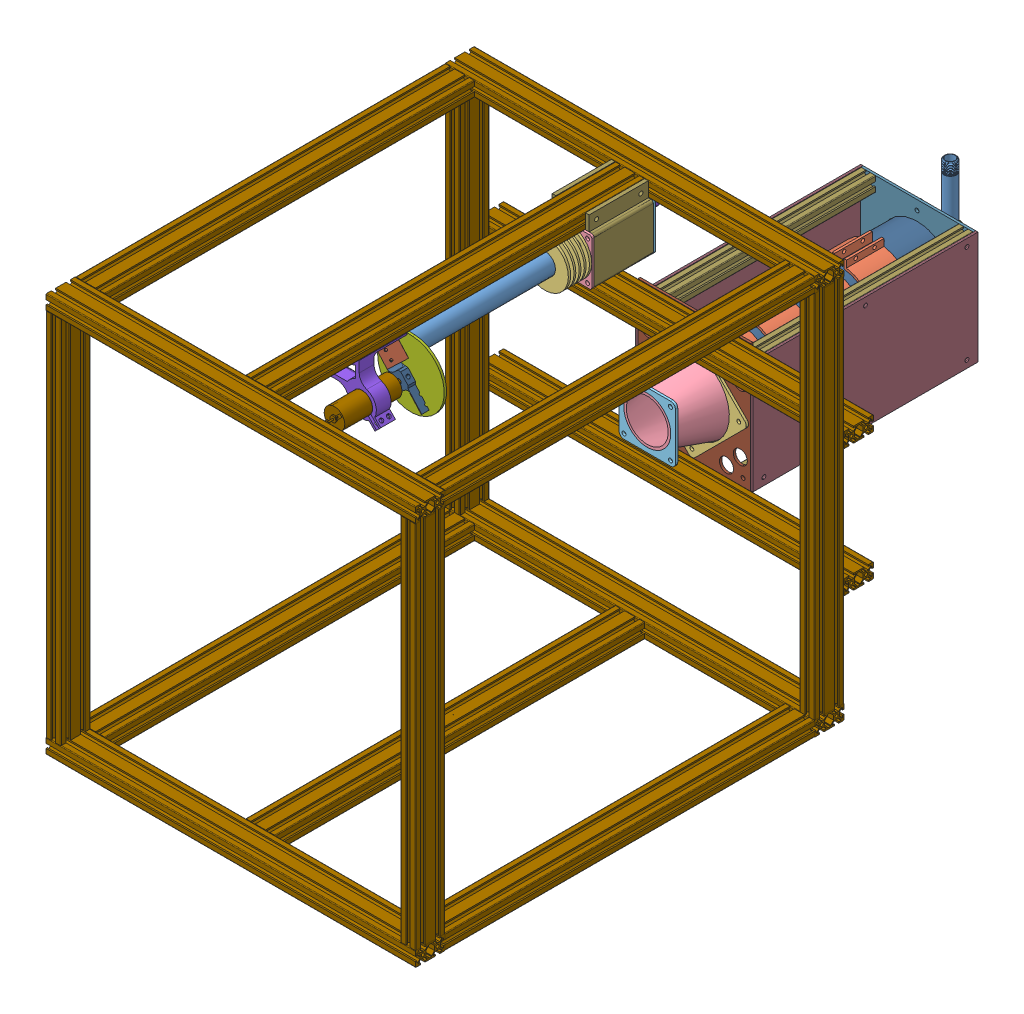
SolidWorks assembly extruder 1 assembly, configuration Default. Lengths in mm.
Overall size (500 540 979.81).
58 component instances, 30 part files, 85 mates.
Components (placement in the parent):
- extruder barrel_rev01-1: extruder barrel_rev01 [Default] at (188.8223 217.5446 43.8354) size (28.57 28.57 304.8)
- nozzle_rev01-1: nozzle_rev01 [Default] at (188.8223 217.5446 329.5854) size (28.57 28.57 31.75)
- barrel lock-1: barrel lock [Default] at (188.8223 217.5446 154.9604) x (-0.997738 -0.067218 0) z (0.067218 -0.997738 0) size (63.5 31.75 63.5)
- barrel lock mount-1: barrel lock mount [Default] at (188.8223 217.5446 120.0354) x (1 0 0) z (0 -1 0) size (63.5 3.17 63.5)
- thrust bearing plate-1: thrust bearing plate [Default] at (188.8223 217.5446 40.0354) x (1 0 0) z (0 1 0) size (63.5 3.17 63.5)
- 5909K310_THRUST NEEDLE-ROLLER BEARING-1: 5909K310_THRUST NEEDLE-ROLLER BEARING [5909K31] at (188.8223 217.5446 42.0304) x (1 0 0) z (0 -1 0) size (23.81 19.84 23.81)
- 5909K440_THRUST NEEDLE-ROLLER BEARING-1: 5909K440_THRUST NEEDLE-ROLLER BEARING [5909K44] at (188.8223 217.5446 41.0382) x (0 0 -1) z (0.082579 0.996584 0) size (0.81 23.81 23.81)
- 5909K440_THRUST NEEDLE-ROLLER BEARING-2: 5909K440_THRUST NEEDLE-ROLLER BEARING [5909K44] at (188.8223 217.5446 43.8354) x (0 0 -1) z (1 0 0) size (0.81 23.81 23.81)
- screw standin-1: screw standin [Default] at (188.8223 217.5446 310.5354) x (1 0 0) z (0 1 0) size (19.55 342.9 19.55)
- 500mm 2040-1: 500mm 2040 [Default] at (188.8223 259.2946 540.0354) x (0 -1 0) z (0 0 1) size (20 40 500)
- 500mm 2040-2: 500mm 2040 [Default] at (-61.3618 259.2946 560.0354) x (0 1 0) z (-1 0 0) size (20 40 500)
- 500mm 2040-3: 500mm 2040 [Default] at (-51.3618 249.2946 560.0354) x (1 0 0) z (0 1 0) size (20 40 500)
- 500mm 2040-4: 500mm 2040 [Default] at (428.6382 -250.7054 560.0354) x (1 0 0) z (0 -1 0) size (20 40 500)
- 500mm 2040-5: 500mm 2040 [Default] at (-61.3618 -260.7054 560.0354) x (0 1 0) z (-1 0 0) size (20 40 500)
- 500mm 2040-6: 500mm 2040 [Default] at (418.6382 259.2946 540.0354) x (0 1 0) z (0 0 1) size (20 40 500)
- 500mm 2040-7: 500mm 2040 [Default] at (-41.3618 259.2946 540.0354) x (0 1 0) z (0 0 1) size (20 40 500)
- 500mm 2040-8: 500mm 2040 [Default] at (418.6382 -260.7054 540.0354) x (0 1 0) z (0 0 1) size (20 40 500)
- 500mm 2040-9: 500mm 2040 [Default] at (-41.3618 -260.7054 540.0354) x (0 -1 0) z (0 0 1) size (20 40 500)
- 500mm 2040-10: 500mm 2040 [Default] at (-61.3618 -260.7054 20.0354) x (0 1 0) z (-1 0 0) size (20 40 500)
- 500mm 2040-11: 500mm 2040 [Default] at (-61.3618 259.2946 20.0354) x (0 -1 0) z (-1 0 0) size (20 40 500)
- 500mm 2040-12: 500mm 2040 [Default] at (-51.3618 249.2946 20.0354) x (-1 0 0) z (0 1 0) size (20 40 500)
- 500mm 2040-13: 500mm 2040 [Default] at (428.6382 249.2946 20.0354) x (1 0 0) z (0 1 0) size (20 40 500)
- 500mm 2040-14: 500mm 2040 [Default] at (188.8164 -260.7054 540.0354) x (0 -1 0) z (0 0 1) size (20 40 500)
- dryer stand alone-1: dryer stand alone [Default] at (381.6192 -132.2091 21.3365) x (0 1 0) z (-1 0 0) size (209.74 423.31 158.7)
  - tube-1: tube [Default] at (103.5422 61.3012 185.6839) size (164.34 304.8 101.6)
  - flange rev01-1: flange rev01 [Default] at (103.5422 61.3012 185.6839) x (-1 0 0) z (0 0 -1) size (192.4 3.17 152.4)
  - HFS5-2020-299-1: HFS5-2020-299 [Default] at (169.7422 63.9262 119.4839) x (-1 0 0) z (0 -1 0) size (20 20 298.45)
  - HFS5-2020-299-2: HFS5-2020-299 [Default] at (37.3422 63.9262 119.4839) x (-1 0 0) z (0 -1 0) size (20 20 298.45)
  - HFS5-2020-299-3: HFS5-2020-299 [Default] at (169.7422 63.9262 251.8839) x (-1 0 0) z (0 -1 0) size (20 20 298.45)
  - HFS5-2020-299-4: HFS5-2020-299 [Default] at (37.3422 363.4762 251.8839) x (-1 0 0) z (0 1 0) size (20 20 298.45)
  - side plate 1_16-1: side plate 1_16 [Default] at (103.5422 213.7012 263.4587) x (-1 0 0) z (0 0 -1) size (152.4 304.8 1.57)
  - side plate 1_16-2: side plate 1_16 [Default] at (103.5422 213.7012 265.0335) x (-1 0 0) z (0 0 -1) size (152.4 304.8 1.57)
  - flange rev02-1: flange rev02 [Default] at (103.5422 362.9262 185.6839) x (-1 0 0) z (0 0 -1) size (152.4 3.17 152.4)
  - top cover-1: top cover [Default] at (103.5422 369.2762 185.6839) x (-0.707107 0 -0.707107) z (0 -1 0) size (107.76 107.76 3.17)
  - 4452K413_TYPE 316 STAINLESS STL THREADED PIPE FITTING-2: 4452K413_TYPE 316 STAINLESS STL THREADED PIPE FITTING [4452K413] at (103.5422 407.8982 185.6839) x (-1 0 0) z (0 0 1) size (37.28 37.03 30.11)
  - 4548K159_STD-WALL TYPE 316-316L SS THRD PIPE NIPPLE-1: 4548K159_STD-WALL TYPE 316-316L SS THRD PIPE NIPPLE [4548K159] at (103.5422 292.6762 185.6839) x (0 1 0) z (0 0 1) size (203.35 17.91 17.78)
  - 4464K498_TYPE 304 STAINLESS STL THREADED PIPE FITTING-1: 4464K498_TYPE 304 STAINLESS STL THREADED PIPE FITTING [4464K498] at (103.5422 180.2482 185.6839) x (-0.837169 0 -0.546944) z (0 1 0) size (25.91 25.91 21.03)
  - 4548K145_STD-WALL TYPE 316-316L SS THRD PIPE NIPPLE-2: 4548K145_STD-WALL TYPE 316-316L SS THRD PIPE NIPPLE [4548K145] at (161.6142 407.8982 185.6839) x (1 0 0) z (0 -0.851872 -0.523749) size (89.04 17.99 18.06)
  - heater band-1: heater band [Default] at (103.5422 257.8762 185.6839) size (116.47 50.8 107.95)
  - heater band-2: heater band [Default] at (103.5422 132.2762 185.6839) size (116.47 50.8 107.95)
  - heater band-3: heater band [Default] at (103.5422 69.4762 185.6839) size (116.47 50.8 107.95)
  - heater band-4: heater band [Default] at (103.5422 195.0762 185.6839) size (116.47 50.8 107.95)
  - bottom cover-1: bottom cover [Default] at (103.6306 61.3012 185.6839) x (-0.707107 0 -0.707107) z (0 -1 0) size (107.76 107.76 3.17)
  - nozzle reduction-1: nozzle reduction [Default] at (103.6306 61.3012 185.6839) x (-0.837169 0 -0.546944) z (-0.546944 0 0.837169) size (101.6 63.5 101.6)
  - 2.5 in bracket-1: 2.5 in bracket [Default] at (103.6306 -2.1988 185.6839) size (76.2 3.17 76.2)
  - side plate 1_16-7: side plate 1_16 [Default] at (103.5422 213.7012 107.9091) size (152.4 304.8 1.57)
  - side plate 1_16-8: side plate 1_16 [Default] at (103.5422 213.7012 106.3343) size (152.4 304.8 1.57)
  - 9157K150_STD-WALL 304-304L SS THRD ONE END PIPE NIPPLE-1: 9157K150_STD-WALL 304-304L SS THRD ONE END PIPE NIPPLE [9157K15] at (103.5422 378.8012 152.0289) x (0 1 0) z (-0.332767 0 0.943009) size (25.49 27.89 27.84)
  - 9157K150_STD-WALL 304-304L SS THRD ONE END PIPE NIPPLE-2: 9157K150_STD-WALL 304-304L SS THRD ONE END PIPE NIPPLE [9157K15] at (103.5422 378.8012 219.3389) x (0 1 0) z (-0.546944 0 0.837169) size (25.49 27.89 27.84)
- pelletizer plate-1: pelletizer plate [Default] at (188.8223 217.5446 361.3354) x (-1 0 0) z (0 -1 0) size (90.17 3.17 90.52)
- pelletizer plate mount-1: pelletizer plate mount [Default] at (188.8223 244.2946 361.3354) x (1 0 0) z (0 -1 0) size (90.17 65 92.21)
- 3262_1-2: 3262_1 [Default] at (212.8568 202.1389 463.8354) x (-0.745096 -0.666957 0) z (0 0 -1) size (28 28 106.2)
- blade wheel-1: blade wheel [Default] at (212.8568 202.1389 366.6354) x (-0.666957 0.745096 0) z (0.745096 0.666957 0) size (76.2 10 20)
- blade fin-1: blade fin [Default] at (229.121 181.0645 369.3692) x (0.570777 0.510919 0.642788) z (-0.666957 0.745096 0) size (23.8 0.5 23.1)
- blade fin-2: blade fin [Default] at (196.3535 222.9985 368.9862) x (-0.570777 -0.510919 0.642788) z (-0.666957 0.745096 0) size (23.8 0.5 23.1)
- hopper rev02-2: hopper rev02 [Default] at (188.8223 217.5446 120.0354) x (1 0 0) z (0 1 0) size (63.5 80 83.5)
- 500mm 2040-16: 500mm 2040 [Default] at (-61.3618 57.5332 -19.9646) x (0 -1 0) z (-1 0 0) size (20 40 500)
- 500mm 2040-17: 500mm 2040 [Default] at (438.6382 -114.8668 -19.9646) x (0 -1 0) z (1 0 0) size (20 40 500)
Mates (geometry in assembly coordinates):
- Concentric1: concentric anti-aligned: cylinder of extruder barrel_rev01-1 through (188.8223 217.5446 329.5854) axis (0 0 1) radius 11.1125; cylinder of nozzle_rev01-1 through (188.8223 217.5446 348.6354) axis (0 0 -1) radius 11.1125
- Coincident1: coincident anti-aligned: plane of extruder barrel_rev01-1 through (188.8223 217.5446 348.6354) normal (0 0 1); plane of nozzle_rev01-1 through (188.8223 217.5446 348.6354) normal (0 0 -1)
- Concentric2: concentric anti-aligned: cylinder of extruder barrel_rev01-1 through (188.8223 217.5446 348.6354) axis (0 0 -1) radius 14.2875; cylinder of barrel lock-1 through (188.8223 217.5446 123.2104) axis (0 0 1) radius 14.3129
- Distance1: distance = 3.175 mm aligned: plane of barrel lock-1 through (188.8223 217.5446 123.2104) normal (0 0 -1); plane of extruder barrel_rev01-1 through (188.8223 217.5446 120.0354) normal (0 0 -1)
- Concentric3: concentric anti-aligned: cylinder of extruder barrel_rev01-1 through (188.8223 217.5446 348.6354) axis (0 0 -1) radius 14.2875; cylinder of barrel lock mount-1 through (188.8223 217.5446 120.0344) axis (0 0 1) radius 14.3129
- Coincident5: coincident anti-aligned: plane of barrel lock-1 through (188.8223 217.5446 123.2104) normal (0 0 -1); plane of barrel lock mount-1 through (188.8223 217.5446 123.2104) normal (0 0 1)
- Concentric4: concentric anti-aligned: cylinder of extruder barrel_rev01-1 through (188.8223 217.5446 348.6354) axis (0 0 -1) radius 9.525; cylinder of 5909K440_THRUST NEEDLE-ROLLER BEARING-2 through (188.8223 217.5446 43.0226) axis (0 0 1) radius 6.3754
- Concentric5: concentric anti-aligned: cylinder of 5909K310_THRUST NEEDLE-ROLLER BEARING-1 through (188.8223 217.5446 41.0382) axis (0 0 -1) radius 6.3754; cylinder of 5909K440_THRUST NEEDLE-ROLLER BEARING-2 through (188.8223 217.5446 43.0226) axis (0 0 1) radius 6.3754
- Tangent1: tangent anti-aligned: cylinder of 5909K310_THRUST NEEDLE-ROLLER BEARING-1 through (195.7165 208.687 42.0304) axis (0.614213 -0.789141 0) radius 0.9922; plane of 5909K440_THRUST NEEDLE-ROLLER BEARING-2 through (188.8223 217.5446 43.0226) normal (0 0 -1)
- Concentric7: concentric anti-aligned: cylinder of 5909K310_THRUST NEEDLE-ROLLER BEARING-1 through (188.8223 217.5446 41.0382) axis (0 0 -1) radius 6.3754; cylinder of 5909K440_THRUST NEEDLE-ROLLER BEARING-1 through (188.8223 217.5446 40.2254) axis (0 0 1) radius 6.3754
- Tangent3: tangent anti-aligned: cylinder of 5909K310_THRUST NEEDLE-ROLLER BEARING-1 through (179.4256 211.4054 42.0304) axis (-0.837166 -0.546948 0) radius 0.9922; plane of 5909K440_THRUST NEEDLE-ROLLER BEARING-1 through (188.8223 217.5446 41.0382) normal (0 0 1)
- Concentric8: concentric anti-aligned: cylinder of extruder barrel_rev01-1 through (188.8223 217.5446 348.6354) axis (0 0 -1) radius 9.525; cylinder of screw standin-1 through (188.8223 217.5446 43.8354) axis (0 0 1) radius 9.525
- Coincident17: coincident anti-aligned: plane of 5909K440_THRUST NEEDLE-ROLLER BEARING-2 through (188.8223 217.5446 43.8354) normal (0 0 1); plane of screw standin-1 through (188.8223 217.5446 43.8354) normal (0 0 -1)
- Coincident18: coincident aligned: plane of barrel lock mount-1 through (220.5723 249.2946 123.2104) normal (0 1 0); plane of thrust bearing plate-1 through (157.0723 249.2946 36.8604) normal (0 1 0)
- Coincident19: coincident aligned: plane of barrel lock mount-1 through (157.0723 185.7946 123.2104) normal (-1 0 0); plane of thrust bearing plate-1 through (157.0723 249.2946 36.8604) normal (-1 0 0)
- Distance2: distance = 80 mm anti-aligned: plane of thrust bearing plate-1 through (188.8223 217.5446 40.0354) normal (0 0 1); plane of barrel lock mount-1 through (188.8223 217.5446 120.0354) normal (0 0 -1)
- Coincident32: coincident aligned: plane of 500mm 2040-1 through (195.8223 269.2946 40.0354) normal (0 1 0); plane of 500mm 2040-2 through (438.6382 269.2946 567.0354) normal (0 1 0)
- Coincident33: coincident anti-aligned: plane of 500mm 2040-1 through (169.8223 268.2946 540.0354) normal (0 0 1); plane of 500mm 2040-2 through (438.6382 256.2946 540.0354) normal (0 0 -1)
- Coincident34: coincident anti-aligned: plane of 500mm 2040-2 through (438.6382 249.2946 553.0354) normal (0 -1 0); plane of 500mm 2040-3 through (-60.3618 249.2946 579.0354) normal (0 1 0)
- Coincident35: coincident aligned: plane of 500mm 2040-2 through (-61.3618 250.2946 579.0354) normal (-1 0 0); plane of 500mm 2040-3 through (-61.3618 -250.7054 553.0354) normal (-1 0 0)
- Coincident36: coincident aligned: plane of 500mm 2040-2 through (438.6382 256.2946 540.0354) normal (0 0 -1); plane of 500mm 2040-3 through (-54.3618 -250.7054 540.0354) normal (0 0 -1)
- Coincident37: coincident anti-aligned: plane of 500mm 2040-2 through (438.6382 249.2946 553.0354) normal (0 -1 0); plane of 500mm 2040-4 through (419.6382 249.2946 541.0354) normal (0 1 0)
- Coincident38: coincident aligned: plane of 500mm 2040-2 through (438.6382 256.2946 540.0354) normal (0 0 -1); plane of 500mm 2040-4 through (431.6382 249.2946 540.0354) normal (0 0 -1)
- Coincident39: coincident aligned: plane of 500mm 2040-2 through (438.6382 250.2946 579.0354) normal (1 0 0); plane of 500mm 2040-4 through (438.6382 249.2946 541.0354) normal (1 0 0)
- Coincident40: coincident anti-aligned: plane of 500mm 2040-3 through (-60.3618 -250.7054 579.0354) normal (0 -1 0); plane of 500mm 2040-5 through (438.6382 -250.7054 567.0354) normal (0 1 0)
- Coincident41: coincident aligned: plane of 500mm 2040-4 through (437.6382 249.2946 580.0354) normal (0 0 1); plane of 500mm 2040-5 through (438.6382 -257.7054 580.0354) normal (0 0 1)
- Coincident42: coincident aligned: plane of 500mm 2040-4 through (438.6382 249.2946 541.0354) normal (1 0 0); plane of 500mm 2040-5 through (438.6382 -269.7054 579.0354) normal (1 0 0)
- Coincident43: coincident anti-aligned: plane of 500mm 2040-2 through (438.6382 256.2946 540.0354) normal (0 0 -1); plane of 500mm 2040-6 through (437.6382 250.2946 540.0354) normal (0 0 1)
- Coincident44: coincident aligned: plane of 500mm 2040-2 through (438.6382 269.2946 567.0354) normal (0 1 0); plane of 500mm 2040-6 through (425.6382 269.2946 40.0354) normal (0 1 0)
- Coincident45: coincident aligned: plane of 500mm 2040-2 through (438.6382 250.2946 579.0354) normal (1 0 0); plane of 500mm 2040-6 through (438.6382 262.2946 40.0354) normal (1 0 0)
- Coincident46: coincident anti-aligned: plane of 500mm 2040-2 through (438.6382 256.2946 540.0354) normal (0 0 -1); plane of 500mm 2040-7 through (-22.3618 250.2946 540.0354) normal (0 0 1)
- Coincident47: coincident aligned: plane of 500mm 2040-2 through (-61.3618 250.2946 579.0354) normal (-1 0 0); plane of 500mm 2040-7 through (-61.3618 268.2946 40.0354) normal (-1 0 0)
- Coincident48: coincident aligned: plane of 500mm 2040-2 through (438.6382 269.2946 547.0354) normal (0 1 0); plane of 500mm 2040-7 through (-34.3618 269.2946 40.0354) normal (0 1 0)
- Coincident49: coincident anti-aligned: plane of 500mm 2040-5 through (438.6382 -251.7054 540.0354) normal (0 0 -1); plane of 500mm 2040-8 through (437.6382 -269.7054 540.0354) normal (0 0 1)
- Coincident50: coincident aligned: plane of 500mm 2040-5 through (438.6382 -269.7054 579.0354) normal (1 0 0); plane of 500mm 2040-8 through (438.6382 -257.7054 40.0354) normal (1 0 0)
- Coincident51: coincident aligned: plane of 500mm 2040-5 through (438.6382 -270.7054 541.0354) normal (0 -1 0); plane of 500mm 2040-8 through (411.6382 -270.7054 40.0354) normal (0 -1 0)
- Coincident52: coincident anti-aligned: plane of 500mm 2040-5 through (438.6382 -251.7054 540.0354) normal (0 0 -1); plane of 500mm 2040-9 through (-60.3618 -251.7054 540.0354) normal (0 0 1)
- Coincident53: coincident aligned: plane of 500mm 2040-5 through (-61.3618 -269.7054 579.0354) normal (-1 0 0); plane of 500mm 2040-9 through (-61.3618 -251.7054 40.0354) normal (-1 0 0)
- Coincident54: coincident aligned: plane of 500mm 2040-5 through (438.6382 -270.7054 541.0354) normal (0 -1 0); plane of 500mm 2040-9 through (-60.3618 -270.7054 40.0354) normal (0 -1 0)
- Coincident55: coincident anti-aligned: plane of 500mm 2040-8 through (437.6382 -269.7054 40.0354) normal (0 0 -1); plane of 500mm 2040-10 through (438.6382 -269.7054 40.0354) normal (0 0 1)
- Coincident56: coincident aligned: plane of 500mm 2040-8 through (438.6382 -257.7054 40.0354) normal (1 0 0); plane of 500mm 2040-10 through (438.6382 -269.7054 39.0354) normal (1 0 0)
- Coincident57: coincident aligned: plane of 500mm 2040-8 through (411.6382 -270.7054 40.0354) normal (0 -1 0); plane of 500mm 2040-10 through (438.6382 -270.7054 33.0354) normal (0 -1 0)
- Coincident58: coincident anti-aligned: plane of 500mm 2040-6 through (437.6382 250.2946 40.0354) normal (0 0 -1); plane of 500mm 2040-11 through (438.6382 262.2946 40.0354) normal (0 0 1)
- Coincident59: coincident aligned: plane of 500mm 2040-6 through (438.6382 262.2946 40.0354) normal (1 0 0); plane of 500mm 2040-11 through (438.6382 268.2946 1.0354) normal (1 0 0)
- Coincident60: coincident aligned: plane of 500mm 2040-6 through (425.6382 269.2946 40.0354) normal (0 1 0); plane of 500mm 2040-11 through (438.6382 269.2946 39.0354) normal (0 1 0)
- Coincident61: coincident aligned: plane of 500mm 2040-7 through (-34.3618 269.2946 40.0354) normal (0 1 0); plane of 500mm 2040-11 through (438.6382 269.2946 27.0354) normal (0 1 0)
- Coincident62: coincident aligned: plane of 500mm 2040-11 through (438.6382 256.2946 0.0354) normal (0 0 -1); plane of 500mm 2040-12 through (-42.3618 -250.7054 0.0354) normal (0 0 -1)
- Coincident63: coincident anti-aligned: plane of 500mm 2040-10 through (438.6382 -250.7054 27.0354) normal (0 1 0); plane of 500mm 2040-12 through (-42.3618 -250.7054 1.0354) normal (0 -1 0)
- Coincident64: coincident aligned: plane of 500mm 2040-10 through (-61.3618 -269.7054 39.0354) normal (-1 0 0); plane of 500mm 2040-12 through (-61.3618 -250.7054 13.0354) normal (-1 0 0)
- Coincident65: coincident aligned: plane of 500mm 2040-11 through (-61.3618 268.2946 1.0354) normal (-1 0 0); plane of 500mm 2040-12 through (-61.3618 -250.7054 13.0354) normal (-1 0 0)
- Coincident66: coincident anti-aligned: plane of 500mm 2040-10 through (438.6382 -250.7054 27.0354) normal (0 1 0); plane of 500mm 2040-13 through (419.6382 -250.7054 39.0354) normal (0 -1 0)
- Coincident67: coincident aligned: plane of 500mm 2040-10 through (438.6382 -269.7054 39.0354) normal (1 0 0); plane of 500mm 2040-13 through (438.6382 -250.7054 27.0354) normal (1 0 0)
- Coincident68: coincident aligned: plane of 500mm 2040-10 through (438.6382 -251.7054 0.0354) normal (0 0 -1); plane of 500mm 2040-13 through (437.6382 -250.7054 0.0354) normal (0 0 -1)
- Coincident69: coincident anti-aligned: plane of 500mm 2040-5 through (438.6382 -251.7054 540.0354) normal (0 0 -1); plane of 500mm 2040-14 through (169.8164 -251.7054 540.0354) normal (0 0 1)
- Coincident70: coincident aligned: plane of 500mm 2040-5 through (438.6382 -270.7054 553.0354) normal (0 -1 0); plane of 500mm 2040-14 through (181.8164 -270.7054 40.0354) normal (0 -1 0)
- Parallel4: parallel anti-aligned: plane of 500mm 2040-11 through (438.6382 256.2946 0.0354) normal (0 0 -1); plane of dryer stand alone-1/2.5 in bracket-1 through (195.9354 -28.5784 23.5354) normal (0 0 1)
- Coincident89: coincident aligned: plane of nozzle_rev01-1 through (188.8223 217.5446 361.3354) normal (0 0 1); plane of pelletizer plate-1 through (188.8223 217.5446 361.3354) normal (0 0 1)
- Coincident90: coincident anti-aligned: plane of 500mm 2040-1 through (181.8223 249.2946 40.0354) normal (0 -1 0); plane of pelletizer plate-1 through (188.8223 249.2946 358.1604) normal (0 1 0)
- Concentric9: concentric anti-aligned: cylinder of nozzle_rev01-1 through (188.8223 217.5446 361.3354) axis (0 0 -1) radius 14.2875; cylinder of pelletizer plate-1 through (188.8223 217.5446 358.1604) axis (0 0 1) radius 13.335
- Coincident91: coincident anti-aligned: plane of 500mm 2040-1 through (181.8223 249.2946 40.0354) normal (0 -1 0); plane of pelletizer plate mount-1 through (168.8223 249.2946 426.3354) normal (0 1 0)
- Coincident92: coincident anti-aligned: plane of pelletizer plate-1 through (188.8223 217.5446 361.3354) normal (0 0 1); plane of pelletizer plate mount-1 through (188.8223 244.2946 361.3354) normal (0 0 -1)
- Coincident93: coincident aligned: plane of 500mm 2040-1 through (168.8223 256.2946 40.0354) normal (-1 0 0); plane of pelletizer plate mount-1 through (168.8223 239.2946 426.3354) normal (-1 0 0)
- Concentric12: concentric aligned: cylinder of 3262_1-2 through (212.8568 202.1389 383.3354) axis (0 0 -1) radius 3; cylinder of blade wheel-1 through (212.8568 202.1389 376.6354) axis (0 0 -1) radius 3.165
- Parallel7: parallel aligned: plane of 3262_1-2 through (214.7276 203.8134 381.3354) normal (0.745096 0.666957 0); plane of blade wheel-1 through (226.9773 201.3575 338.3511) normal (0.745096 0.666957 0)
- Parallel8: parallel anti-aligned: plane of 3262_1-2 through (212.8568 202.1389 384.3354) normal (0 0 -1); plane of blade wheel-1 through (212.8568 202.1389 376.6354) normal (0 0 1)
- Coincident96: coincident aligned: plane of 3262_1-2 through (212.9764 202.2459 366.6354) normal (0 0 -1); plane of blade wheel-1 through (212.8568 202.1389 366.6354) normal (0 0 -1)
- Distance3: distance = 20 mm aligned: plane of 3262_1-2 through (212.8568 202.1389 386.3354) normal (0 0 -1); plane of pelletizer plate mount-1 through (212.9094 202.1712 406.3354) normal (0 0 -1)
- Coincident100: coincident anti-aligned: plane of blade wheel-1 through (225.1146 199.6901 376.6354) normal (-0.478938 -0.428712 0.766044); plane of blade fin-1 through (229.3605 181.2788 368.9862) normal (0.478938 0.428712 -0.766044)
- Coincident101: coincident aligned: plane of blade wheel-1 through (243.8561 178.7529 376.6354) normal (0.666957 -0.745096 0); plane of blade fin-1 through (230.2716 166.593 361.337) normal (0.666957 -0.745096 0)
- Coincident102: coincident: line of blade wheel-1 through (243.8561 178.7529 376.6354) axis (-0.666957 0.745096 0); plane of blade fin-1 through (243.8561 178.7529 376.6354) normal (0.570777 0.510919 0.642788)
- Coincident103: coincident anti-aligned: plane of blade wheel-1 through (200.599 204.5876 376.6354) normal (0.478938 0.428712 0.766044); plane of blade fin-2 through (196.3535 222.9985 368.9862) normal (-0.478938 -0.428712 -0.766044)
- Concentric13: concentric aligned: cylinder of blade wheel-1 through (185.8603 221.0544 364.5351) axis (0.478938 0.428712 0.766044) radius 2.5; cylinder of blade fin-2 through (190.299 225.0276 371.6346) axis (0.478938 0.428712 0.766044) radius 1.665
- Concentric14: concentric aligned: cylinder of blade wheel-1 through (193.2631 212.7843 364.5351) axis (0.478938 0.428712 0.766044) radius 2.5; cylinder of blade fin-2 through (197.7019 216.7575 371.6346) axis (0.478938 0.428712 0.766044) radius 1.665
- Coincident104: coincident anti-aligned: plane of barrel lock mount-1 through (188.8223 217.5446 120.0354) normal (0 0 -1); plane of hopper rev02-2 through (188.8223 217.5446 120.0354) normal (0 0 1)
- Coincident105: coincident aligned: plane of barrel lock mount-1 through (220.5723 185.7946 123.2104) normal (1 0 0); plane of hopper rev02-2 through (220.5723 185.7946 40.0354) normal (1 0 0)
- Coincident106: coincident aligned: plane of barrel lock mount-1 through (220.5723 185.7946 123.2104) normal (0 -1 0); plane of hopper rev02-2 through (157.0723 185.7946 40.0354) normal (0 -1 0)
- Coincident114: coincident anti-aligned: plane of 500mm 2040-13 through (437.6382 -250.7054 0.0354) normal (0 0 -1); plane of 500mm 2040-16 through (438.6382 48.5332 0.0354) normal (0 0 1)
- Coincident116: coincident aligned: plane of 500mm 2040-13 through (438.6382 -250.7054 27.0354) normal (1 0 0); plane of 500mm 2040-16 through (438.6382 66.5332 -38.9646) normal (1 0 0)
- Coincident117: coincident anti-aligned: plane of dryer stand alone-1/flange rev01-1 through (195.9354 -28.6668 -39.9646) normal (0 0 1); plane of 500mm 2040-16 through (438.6382 54.5332 -39.9646) normal (0 0 -1)
- Coincident118: coincident aligned: plane of dryer stand alone-1/flange rev01-1 through (195.9354 67.5332 -39.9646) normal (0 1 0); plane of 500mm 2040-16 through (438.6382 67.5332 -32.9646) normal (0 1 0)
- Coincident119: coincident anti-aligned: plane of 500mm 2040-1 through (208.8223 262.2946 40.0354) normal (1 0 0); plane of hopper rev02-2 through (208.8223 269.2946 40.0354) normal (-1 0 0)
- Coincident120: coincident anti-aligned: plane of 500mm 2040-12 through (-42.3618 -250.7054 0.0354) normal (0 0 -1); plane of 500mm 2040-17 through (-61.3618 -117.8668 0.0354) normal (0 0 1)
- Coincident121: coincident aligned: plane of 500mm 2040-12 through (-61.3618 -250.7054 13.0354) normal (-1 0 0); plane of 500mm 2040-17 through (-61.3618 -105.8668 -0.9646) normal (-1 0 0)
- Coincident122: coincident aligned: plane of dryer stand alone-1/flange rev01-1 through (195.9354 -124.8668 -39.9646) normal (0 -1 0); plane of 500mm 2040-17 through (-61.3618 -124.8668 -12.9646) normal (0 -1 0)
- Coincident123: coincident anti-aligned: plane of 500mm 2040-11 through (438.6382 262.2946 40.0354) normal (0 0 1); plane of hopper rev02-2 through (188.8223 217.5446 40.0354) normal (0 0 -1)
